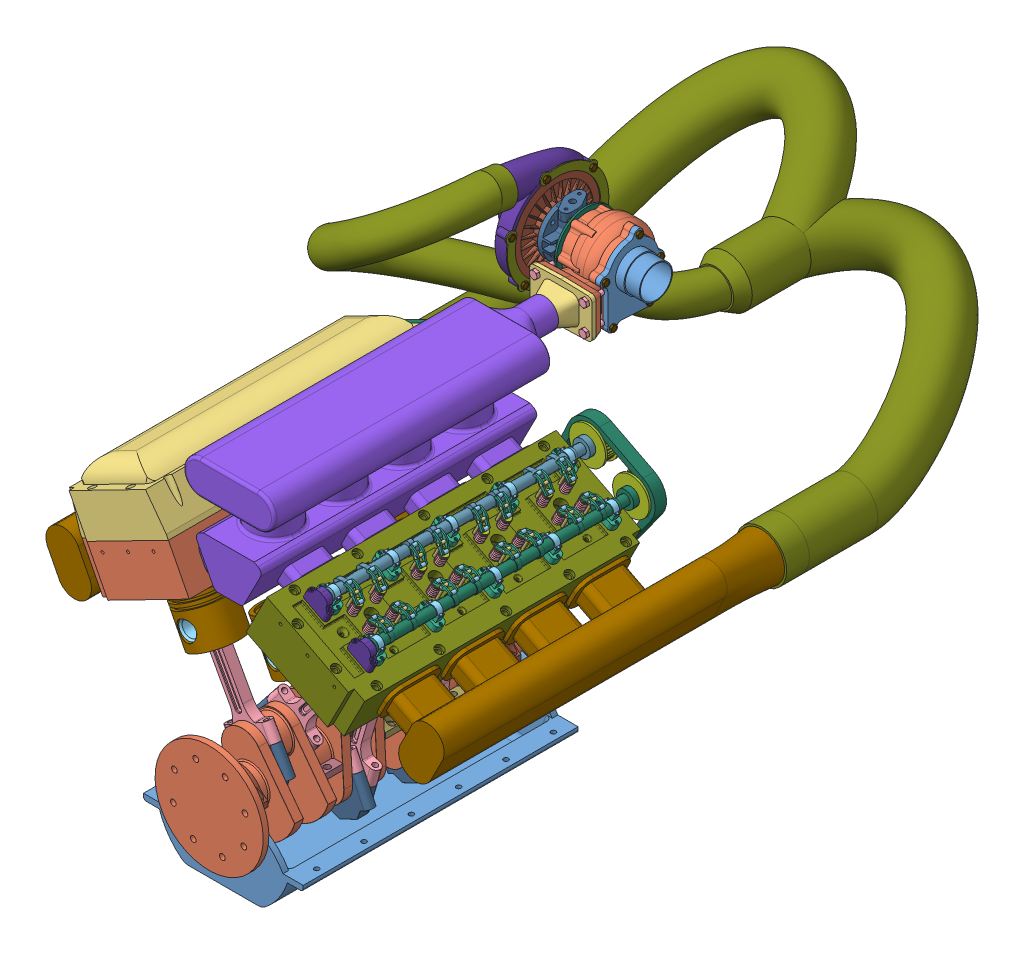
SolidWorks assembly ENSAMBLAJE DE MOTOR V8, configuration Predeterminado. Lengths in mm. (continued)
Components (placement in the parent): (continued)
- CUBIERTA DE SOPORTE DE ARBOL DE LEVAS-14: CUBIERTA DE SOPORTE DE ARBOL DE LEVAS [Predeterminado] at (198.243 212.1897 690.5) x (0.890111 -0.455744 0) z (0 0 1) size (25 9.96 10)
- SOPORTE DE ARBOL DE LEVAS-14: SOPORTE DE ARBOL DE LEVAS [Predeterminado] at (173.0848 200.3549 695.5) x (0.890111 -0.455744 0) z (0 0 1) size (40.64 22 18)
- CUBIERTA DE SOPORTE DE ARBOL DE LEVAS-15: CUBIERTA DE SOPORTE DE ARBOL DE LEVAS [Predeterminado] at (-150.1483 251.4202 398.25) x (0.890111 0.455744 0) z (0 0 1) size (25 9.96 10)
- SOPORTE DE ARBOL DE LEVAS-15: SOPORTE DE ARBOL DE LEVAS [Predeterminado] at (-155.2538 224.0901 403.25) x (0.890111 0.455744 0) z (0 0 1) size (40.64 22 18)
- CUBIERTA DE SOPORTE DE ARBOL DE LEVAS-16: CUBIERTA DE SOPORTE DE ARBOL DE LEVAS [Predeterminado] at (198.243 212.1897 587.5) x (0.890111 -0.455744 0) z (0 0 1) size (25 9.96 10)
- SOPORTE DE ARBOL DE LEVAS-16: SOPORTE DE ARBOL DE LEVAS [Predeterminado] at (173.0848 200.3549 592.5) x (0.890111 -0.455744 0) z (0 0 1) size (40.64 22 18)
- CUBIERTA DE SOPORTE DE ARBOL DE LEVAS-17: CUBIERTA DE SOPORTE DE ARBOL DE LEVAS [Predeterminado] at (121.6935 251.3837 690.5) x (0.890111 -0.455744 0) z (0 0 1) size (25 9.96 10)
- SOPORTE DE ARBOL DE LEVAS-17: SOPORTE DE ARBOL DE LEVAS [Predeterminado] at (96.5352 239.5489 695.5) x (0.890111 -0.455744 0) z (0 0 1) size (40.64 22 18)
- CUBIERTA DE SOPORTE DE ARBOL DE LEVAS-18: CUBIERTA DE SOPORTE DE ARBOL DE LEVAS [Predeterminado] at (198.243 212.1897 484.5) x (0.890111 -0.455744 0) z (0 0 1) size (25 9.96 10)
- SOPORTE DE ARBOL DE LEVAS-18: SOPORTE DE ARBOL DE LEVAS [Predeterminado] at (173.0848 200.3549 489.5) x (0.890111 -0.455744 0) z (0 0 1) size (40.64 22 18)
- CUBIERTA DE SOPORTE DE ARBOL DE LEVAS-19: CUBIERTA DE SOPORTE DE ARBOL DE LEVAS [Predeterminado] at (121.6935 251.3837 484.5) x (0.890111 -0.455744 0) z (0 0 1) size (25 9.96 10)
- SOPORTE DE ARBOL DE LEVAS-19: SOPORTE DE ARBOL DE LEVAS [Predeterminado] at (96.5352 239.5489 489.5) x (0.890111 -0.455744 0) z (0 0 1) size (40.64 22 18)
- CUBIERTA DE SOPORTE DE ARBOL DE LEVAS-20: CUBIERTA DE SOPORTE DE ARBOL DE LEVAS [Predeterminado] at (121.6935 251.3837 587.5) x (0.890111 -0.455744 0) z (0 0 1) size (25 9.96 10)
- SOPORTE DE ARBOL DE LEVAS-20: SOPORTE DE ARBOL DE LEVAS [Predeterminado] at (96.5352 239.5489 592.5) x (0.890111 -0.455744 0) z (0 0 1) size (40.64 22 18)
- CUBIERTA DE SOPORTE DE ARBOL DE LEVAS-21: CUBIERTA DE SOPORTE DE ARBOL DE LEVAS [Predeterminado] at (198.243 212.1897 278.5) x (0.890111 -0.455744 0) z (0 0 1) size (25 9.96 10)
- SOPORTE DE ARBOL DE LEVAS-21: SOPORTE DE ARBOL DE LEVAS [Predeterminado] at (173.0848 200.3549 283.5) x (0.890111 -0.455744 0) z (0 0 1) size (40.64 22 18)
- CUBIERTA DE SOPORTE DE ARBOL DE LEVAS-22: CUBIERTA DE SOPORTE DE ARBOL DE LEVAS [Predeterminado] at (198.243 212.1897 381.5) x (0.890111 -0.455744 0) z (0 0 1) size (25 9.96 10)
- SOPORTE DE ARBOL DE LEVAS-22: SOPORTE DE ARBOL DE LEVAS [Predeterminado] at (173.0848 200.3549 386.5) x (0.890111 -0.455744 0) z (0 0 1) size (40.64 22 18)
- CUBIERTA DE SOPORTE DE ARBOL DE LEVAS-23: CUBIERTA DE SOPORTE DE ARBOL DE LEVAS [Predeterminado] at (121.6935 251.3837 381.5) x (0.890111 -0.455744 0) z (0 0 1) size (25 9.96 10)
- SOPORTE DE ARBOL DE LEVAS-23: SOPORTE DE ARBOL DE LEVAS [Predeterminado] at (96.5352 239.5489 386.5) x (0.890111 -0.455744 0) z (0 0 1) size (40.64 22 18)
- CUBIERTA DE SOPORTE DE ARBOL DE LEVAS-24: CUBIERTA DE SOPORTE DE ARBOL DE LEVAS [Predeterminado] at (121.6935 251.3837 278.5) x (0.890111 -0.455744 0) z (0 0 1) size (25 9.96 10)
- SOPORTE DE ARBOL DE LEVAS-24: SOPORTE DE ARBOL DE LEVAS [Predeterminado] at (96.5352 239.5489 283.5) x (0.890111 -0.455744 0) z (0 0 1) size (40.64 22 18)
- CUBIERTA DE SOPORTE DE ARBOL DE LEVAS-25: CUBIERTA DE SOPORTE DE ARBOL DE LEVAS [Predeterminado] at (-150.1483 251.4202 612.25) x (0.890111 0.455744 0) z (0 0 1) size (25 9.96 10)
- SOPORTE DE ARBOL DE LEVAS-25: SOPORTE DE ARBOL DE LEVAS [Predeterminado] at (-155.2538 224.0901 617.25) x (0.890111 0.455744 0) z (0 0 1) size (40.64 22 18)
- CUBIERTA DE SOPORTE DE ARBOL DE LEVAS-26: CUBIERTA DE SOPORTE DE ARBOL DE LEVAS [Predeterminado] at (-150.1483 251.4202 291.25) x (0.890111 0.455744 0) z (0 0 1) size (25 9.96 10)
- SOPORTE DE ARBOL DE LEVAS-26: SOPORTE DE ARBOL DE LEVAS [Predeterminado] at (-231.8033 184.8961 617.25) x (0.890111 0.455744 0) z (0 0 1) size (40.64 22 18)
- CUBIERTA DE SOPORTE DE ARBOL DE LEVAS-27: CUBIERTA DE SOPORTE DE ARBOL DE LEVAS [Predeterminado] at (-226.6978 212.2262 612.25) x (0.890111 0.455744 0) z (0 0 1) size (25 9.96 10)
- SOPORTE DE ARBOL DE LEVAS-27: SOPORTE DE ARBOL DE LEVAS [Predeterminado] at (-155.2538 224.0901 716.25) x (0.890111 0.455744 0) z (0 0 1) size (40.64 22 18)
- CUBIERTA DE SOPORTE DE ARBOL DE LEVAS-28: CUBIERTA DE SOPORTE DE ARBOL DE LEVAS [Predeterminado] at (-226.6978 212.2262 505.25) x (0.890111 0.455744 0) z (0 0 1) size (25 9.96 10)
- SOPORTE DE ARBOL DE LEVAS-28: SOPORTE DE ARBOL DE LEVAS [Predeterminado] at (-231.8033 184.8961 510.25) x (0.890111 0.455744 0) z (0 0 1) size (40.64 22 18)
- CUBIERTA DE SOPORTE DE ARBOL DE LEVAS-29: CUBIERTA DE SOPORTE DE ARBOL DE LEVAS [Predeterminado] at (-226.6978 212.2262 711.25) x (0.890111 0.455744 0) z (0 0 1) size (25 9.96 10)
- SOPORTE DE ARBOL DE LEVAS-29: SOPORTE DE ARBOL DE LEVAS [Predeterminado] at (-231.8033 184.8961 716.25) x (0.890111 0.455744 0) z (0 0 1) size (40.64 22 18)
- CUBIERTA DE SOPORTE DE ARBOL DE LEVAS-30: CUBIERTA DE SOPORTE DE ARBOL DE LEVAS [Predeterminado] at (-150.1483 251.4202 505.25) x (0.890111 0.455744 0) z (0 0 1) size (25 9.96 10)
- SOPORTE DE ARBOL DE LEVAS-30: SOPORTE DE ARBOL DE LEVAS [Predeterminado] at (-155.2538 224.0901 510.25) x (0.890111 0.455744 0) z (0 0 1) size (40.64 22 18)
- CUBIERTA DE SOPORTE DE ARBOL DE LEVAS-31: CUBIERTA DE SOPORTE DE ARBOL DE LEVAS [Predeterminado] at (-150.1483 251.4202 711.25) x (0.890111 0.455744 0) z (0 0 1) size (25 9.96 10)
- SOPORTE DE ARBOL DE LEVAS-31: SOPORTE DE ARBOL DE LEVAS [Predeterminado] at (-155.2538 224.0901 296.25) x (0.890111 0.455744 0) z (0 0 1) size (40.64 22 18)
- CUBIERTA DE SOPORTE DE ARBOL DE LEVAS-32: CUBIERTA DE SOPORTE DE ARBOL DE LEVAS [Predeterminado] at (-226.6978 212.2262 291.25) x (0.890111 0.455744 0) z (0 0 1) size (25 9.96 10)
- SOPORTE DE ARBOL DE LEVAS-32: SOPORTE DE ARBOL DE LEVAS [Predeterminado] at (-231.8033 184.8961 296.25) x (0.890111 0.455744 0) z (0 0 1) size (40.64 22 18)
- CUBIERTA DE SOPORTE DE ARBOL DE LEVAS-33: CUBIERTA DE SOPORTE DE ARBOL DE LEVAS [Predeterminado] at (-226.6978 212.2262 398.25) x (0.890111 0.455744 0) z (0 0 1) size (25 9.96 10)
- SOPORTE DE ARBOL DE LEVAS-33: SOPORTE DE ARBOL DE LEVAS [Predeterminado] at (-231.8033 184.8961 403.25) x (0.890111 0.455744 0) z (0 0 1) size (40.64 22 18)
- ENGRANE ARBOL DE LEVAS-1: ENGRANE ARBOL DE LEVAS [Predeterminado] at (198.243 212.1897 225) x (0.628385 0.777902 0) z (0 0 1) size (64 64 27)
- ENGRANE CIGUEÑAL-1: ENGRANE CIGUEÑAL [Predeterminado] at (-14.263 -103.8973 245) x (0.937671 0.347525 0) z (0 0 -1) size (30 30 27)
- ENGRANE ARBOL DE LEVAS-2: ENGRANE ARBOL DE LEVAS [Predeterminado] at (121.6935 251.3837 225) x (0.282857 0.959162 0) z (0 0 1) size (64 64 27)
- ENGRANE ARBOL DE LEVAS-3: ENGRANE ARBOL DE LEVAS [Predeterminado] at (-150.1483 251.4202 225) x (-0.43783 0.899058 0) z (0 0 1) size (64 64 27)
- ENGRANE ARBOL DE LEVAS-4: ENGRANE ARBOL DE LEVAS [Predeterminado] at (-226.6978 212.2262 225) x (0.028509 0.999594 0) z (0 0 1) size (64 64 27)
- TORNILLO CABEZA HEXAGONAL_ENGRANE DE ARBOL DE LEVAS-1: TORNILLO CABEZA HEXAGONAL_ENGRANE DE ARBOL DE LEVAS [Predeterminado] at (198.243 212.1897 221.5) size (18 18 59)
- TORNILLO CABEZA HEXAGONAL_ENGRANE DE ARBOL DE LEVAS-2: TORNILLO CABEZA HEXAGONAL_ENGRANE DE ARBOL DE LEVAS [Predeterminado] at (121.6935 251.3837 221.5) size (18 18 59)
- TORNILLO CABEZA HEXAGONAL_ENGRANE DE ARBOL DE LEVAS-3: TORNILLO CABEZA HEXAGONAL_ENGRANE DE ARBOL DE LEVAS [Predeterminado] at (-226.6978 212.2262 221.5) size (18 18 59)
- TORNILLO CABEZA HEXAGONAL_ENGRANE DE ARBOL DE LEVAS-4: TORNILLO CABEZA HEXAGONAL_ENGRANE DE ARBOL DE LEVAS [Predeterminado] at (-150.1483 251.4202 221.5) size (18 18 59)
- TORNILLO CABEZA HEXAGONAL_ENGRANE DE ARBOL DE CIGÜEÑAL-1: TORNILLO CABEZA HEXAGONAL_ENGRANE DE ARBOL DE CIGÜEÑAL [Predeterminado] at (-14.263 -103.8973 221.5) size (20 20 38)
- SOPORTE DE RODAMIENTO PARA LA BANDA-1: SOPORTE DE RODAMIENTO PARA LA BANDA [Predeterminado] at (-14.263 120.8016 248.5) x (0.866025 -0.5 0) z (0 0 1) size (80 80 35.5)
- PERNO HEXAGONAL HUECO_PARA SOPORTE DE RODAMIENTO DE BANDA-1: PERNO HEXAGONAL HUECO_PARA SOPORTE DE RODAMIENTO DE BANDA [Predeterminado] at (7.3876 133.3016 253.5) x (-0.923728 -0.383049 0) z (0 0 -1) size (17.8 17.8 27.6)
- PERNO HEXAGONAL HUECO_PARA SOPORTE DE RODAMIENTO DE BANDA-2: PERNO HEXAGONAL HUECO_PARA SOPORTE DE RODAMIENTO DE BANDA [Predeterminado] at (7.3876 108.3016 253.5) x (-0.793594 0.608447 0) z (0 0 -1) size (17.8 17.8 27.6)
- PERNO HEXAGONAL HUECO_PARA SOPORTE DE RODAMIENTO DE BANDA-3: PERNO HEXAGONAL HUECO_PARA SOPORTE DE RODAMIENTO DE BANDA [Predeterminado] at (-14.263 95.8016 253.5) x (0.130134 0.991496 0) z (0 0 -1) size (17.8 17.8 27.6)
- PERNO HEXAGONAL HUECO_PARA SOPORTE DE RODAMIENTO DE BANDA-4: PERNO HEXAGONAL HUECO_PARA SOPORTE DE RODAMIENTO DE BANDA [Predeterminado] at (-35.9136 108.3016 253.5) x (0.923728 0.383049 0) z (0 0 -1) size (17.8 17.8 27.6)
- PERNO HEXAGONAL HUECO_PARA SOPORTE DE RODAMIENTO DE BANDA-5: PERNO HEXAGONAL HUECO_PARA SOPORTE DE RODAMIENTO DE BANDA [Predeterminado] at (-35.9136 133.3016 253.5) x (0.793594 -0.608447 0) z (0 0 -1) size (17.8 17.8 27.6)
- PERNO HEXAGONAL HUECO_PARA SOPORTE DE RODAMIENTO DE BANDA-6: PERNO HEXAGONAL HUECO_PARA SOPORTE DE RODAMIENTO DE BANDA [Predeterminado] at (-14.263 145.8016 253.5) x (-0.130134 -0.991496 0) z (0 0 -1) size (17.8 17.8 27.6)
- RODAMIENTO DE BANDA-1: RODAMIENTO DE BANDA [Predeterminado] at (-14.263 120.8016 228.5) size (55 55 24.5)
- TORNILLO CABEZA HEXAGONAL_RODAMIENTO-1: TORNILLO CABEZA HEXAGONAL_RODAMIENTO [Predeterminado] at (-14.263 120.8016 224) size (20 20 19)
- BANDA DE DISTRIBUCIÓN-1: BANDA DE DISTRIBUCIÓN [Predeterminado] at (-14.2352 120.7828 235) x (1 -0.000086 0) z (0 0 1) size (502.94 419.82 20)
- RECOLECTOR DE GASES DE ESCAPE-2: RECOLECTOR DE GASES DE ESCAPE [Predeterminado] at origin size (704.57 462.45 809.42)
Mates (geometry in assembly coordinates):
- Concéntrica1: concentric: cylinder of CIGUEÑAL-1 through (-14.263 -103.8973 253.5) axis (0 0 1) radius 32; cylinder of ? through (-14.263 -103.8973 278.5) axis (0 0 -1) radius 32
- Concéntrica9: concentric: cylinder of ? through (-29.5541 -62.6398 627.75) axis (0 0 -1) radius 33; cylinder of COJINETE SUPERIOR-1 through (-29.5541 -62.6398 627.75) axis (0 0 -1) radius 33
- Coincidente2: coincident: plane of ? through (76.4856 71.7664 609.75) normal (0 0 -1); plane of COJINETE SUPERIOR-1 through (-29.5541 -62.6398 609.75) normal (0 0 -1)
- Concéntrica10: concentric: cylinder of ? through (-29.5541 -62.6398 627.75) axis (0 0 -1) radius 33; cylinder of COJINETE INFERIOR-1 through (-29.5541 -62.6398 609.75) axis (0 0 1) radius 32
- Coincidente3: coincident: plane of assembly; plane of assembly; plane of COJINETE INFERIOR-1 through (-0.1804 -77.6794 609.75) normal (-0.455744 -0.890111 0); plane of COJINETE SUPERIOR-1 through (-58.0376 -48.056 627.75) normal (0.455744 0.890111 0)
- Coincidente4: coincident: plane of ? through (76.4856 71.7664 627.75) normal (0 0 1); plane of COJINETE INFERIOR-1 through (-29.5541 -62.6398 627.75) normal (0 0 1)
- Concéntrica11: concentric: cylinder of ? through (76.4856 71.7664 637.75) axis (0 0 -1) radius 17.8; cylinder of COJINETE-1 through (76.4856 71.7664 635.25) axis (0 0 -1) radius 17.8
- Ancho1: width: plane of ? through (76.4856 71.7664 599.75) normal (0 0 -1); plane of ? through (76.4856 71.7664 637.75) normal (0 0 1); plane of COJINETE-1 through (76.4856 71.7664 602.25) normal (0 0 -1); plane of COJINETE-1 through (76.4856 71.7664 635.25) normal (0 0 1)
- Concéntrica12: concentric: cylinder of ? through (76.4856 71.7664 656.65) axis (0 0 -1) radius 16.9; cylinder of COJINETE-1 through (76.4856 71.7664 635.25) axis (0 0 -1) radius 16.9
- Concéntrica13: concentric: cylinder of ? through (84.7286 82.2145 618.75) axis (0.61939 0.785083 0) radius 1.25; cylinder of ? through (74.0699 68.7046 618.75) axis (0.61939 0.785083 0) radius 6.3
- Concéntrica14: concentric: cylinder of ? through (76.4856 71.7664 656.65) axis (0 0 -1) radius 16.9; cylinder of PISTÓN-1 through (76.4856 71.7664 654.5) axis (0 0 -1) radius 16.9
- Ancho2: width: plane of PISTÓN-1 through (67.3727 111.2594 599.75) normal (0 0 1); plane of PISTÓN-1 through (67.3727 111.2594 637.75) normal (0 0 -1); plane of ? through (76.4856 71.7664 599.75) normal (0 0 -1); plane of ? through (76.4856 71.7664 637.75) normal (0 0 1)
- Concéntrica15: concentric: cylinder of assembly; cylinder of assembly; cylinder of COJINETE SUPERIOR-1 through (-29.5541 -62.6398 627.75) axis (0 0 -1) radius 33; cylinder of SOMBRERETE DE BIELA-1 through (-29.5541 -62.6398 600.25) axis (0 0 1) radius 33
- Coincidente5: coincident: plane of ? through (76.4856 71.7664 627.75) normal (0 0 1); plane of SOMBRERETE DE BIELA-1 through (-29.5541 -62.6398 627.75) normal (0 0 1)
- Coincidente6: coincident: plane of ? through (75.9097 72.2187 331.75) normal (0 0 1); plane of COJINETE INFERIOR-2 through (-29.5541 -62.6398 331.75) normal (0 0 1)
- Concéntrica16: concentric: cylinder of ? through (-29.5541 -62.6398 331.75) axis (0 0 -1) radius 33; cylinder of COJINETE INFERIOR-2 through (-29.5541 -62.6398 313.75) axis (0 0 1) radius 32
- Ancho3: width: plane of ? through (75.9097 72.2187 303.75) normal (0 0 -1); plane of ? through (75.9097 72.2187 341.75) normal (0 0 1); plane of COJINETE-2 through (75.9097 72.2187 306.25) normal (0 0 -1); plane of COJINETE-2 through (75.9097 72.2187 339.25) normal (0 0 1)
- Concéntrica17: concentric: cylinder of ? through (75.9097 72.2187 360.65) axis (0 0 -1) radius 16.9; cylinder of PISTÓN-2 through (75.9097 72.2187 358.5) axis (0 0 -1) radius 16.9
- Concéntrica18: concentric: cylinder of ? through (75.9097 72.2187 360.65) axis (0 0 -1) radius 16.9; cylinder of COJINETE-2 through (75.9097 72.2187 339.25) axis (0 0 -1) radius 16.9
- Concéntrica19: concentric: cylinder of ? through (-29.5541 -62.6398 331.75) axis (0 0 -1) radius 33; cylinder of COJINETE SUPERIOR-2 through (-29.5541 -62.6398 331.75) axis (0 0 -1) radius 33
- Concéntrica20: concentric: cylinder of ? through (84.108 82.702 322.75) axis (0.616027 0.787725 0) radius 1.25; cylinder of ? through (73.5072 69.1466 322.75) axis (0.616027 0.787725 0) radius 6.3
- Concéntrica21: concentric: cylinder of ? through (75.9097 72.2187 341.75) axis (0 0 -1) radius 17.8; cylinder of COJINETE-2 through (75.9097 72.2187 339.25) axis (0 0 -1) radius 17.8
- Ancho4: width: plane of PISTÓN-2 through (66.7969 111.7117 303.75) normal (0 0 1); plane of PISTÓN-2 through (66.7969 111.7117 341.75) normal (0 0 -1); plane of ? through (75.9097 72.2187 303.75) normal (0 0 -1); plane of ? through (75.9097 72.2187 341.75) normal (0 0 1)
- Coincidente7: coincident: plane of ? through (75.9097 72.2187 331.75) normal (0 0 1); plane of SOMBRERETE DE BIELA-2 through (-29.5541 -62.6398 331.75) normal (0 0 1)
- Coincidente8: coincident: plane of assembly; plane of assembly; plane of COJINETE INFERIOR-2 through (-0.1804 -77.6794 313.75) normal (-0.455744 -0.890111 0); plane of COJINETE SUPERIOR-2 through (-58.0376 -48.056 331.75) normal (0.455744 0.890111 0)
- Coincidente9: coincident: plane of ? through (75.9097 72.2187 313.75) normal (0 0 -1); plane of COJINETE SUPERIOR-2 through (-29.5541 -62.6398 313.75) normal (0 0 -1)
- Concéntrica22: concentric: cylinder of assembly; cylinder of assembly; cylinder of COJINETE SUPERIOR-2 through (-29.5541 -62.6398 331.75) axis (0 0 -1) radius 33; cylinder of SOMBRERETE DE BIELA-2 through (-29.5541 -62.6398 304.25) axis (0 0 1) radius 33
- Coincidente10: coincident: plane of ? through (-72.3378 9.5283 463.25) normal (0 0 1); plane of COJINETE INFERIOR-3 through (1.0281 -145.1549 463.25) normal (0 0 1)
- Concéntrica23: concentric: cylinder of ? through (1.0281 -145.1549 463.25) axis (0 0 -1) radius 33; cylinder of COJINETE INFERIOR-3 through (1.0281 -145.1549 445.25) axis (0 0 1) radius 32
- Ancho5: width: plane of ? through (-72.3378 9.5283 435.25) normal (0 0 -1); plane of ? through (-72.3378 9.5283 473.25) normal (0 0 1); plane of COJINETE-3 through (-72.3378 9.5283 437.75) normal (0 0 -1); plane of COJINETE-3 through (-72.3378 9.5283 470.75) normal (0 0 1)
- Concéntrica24: concentric: cylinder of ? through (-72.3378 9.5283 492.15) axis (0 0 -1) radius 16.9; cylinder of PISTÓN-3 through (-72.3378 9.5283 490) axis (0 0 -1) radius 16.9
- Concéntrica25: concentric: cylinder of ? through (-72.3378 9.5283 492.15) axis (0 0 -1) radius 16.9; cylinder of COJINETE-3 through (-72.3378 9.5283 470.75) axis (0 0 -1) radius 16.9
- Concéntrica26: concentric: cylinder of ? through (1.0281 -145.1549 463.25) axis (0 0 -1) radius 33; cylinder of COJINETE SUPERIOR-3 through (1.0281 -145.1549 463.25) axis (0 0 -1) radius 33
- Concéntrica27: concentric: cylinder of ? through (-78.0409 21.5527 454.25) axis (-0.428539 0.903523 0) radius 1.25; cylinder of ? through (-70.6665 6.0046 454.25) axis (-0.428539 0.903523 0) radius 6.3
- Concéntrica28: concentric: cylinder of ? through (-72.3378 9.5283 473.25) axis (0 0 -1) radius 17.8; cylinder of COJINETE-3 through (-72.3378 9.5283 470.75) axis (0 0 -1) radius 17.8
- Ancho6: width: plane of PISTÓN-3 through (-109.7068 25.2222 435.25) normal (0 0 1); plane of PISTÓN-3 through (-109.7068 25.2222 473.25) normal (0 0 -1); plane of ? through (-72.3378 9.5283 435.25) normal (0 0 -1); plane of ? through (-72.3378 9.5283 473.25) normal (0 0 1)
- Coincidente11: coincident: plane of ? through (-72.3378 9.5283 463.25) normal (0 0 1); plane of SOMBRERETE DE BIELA-3 through (1.0281 -145.1549 463.25) normal (0 0 1)
- Coincidente12: coincident: plane of assembly; plane of assembly; plane of COJINETE INFERIOR-3 through (30.4018 -130.1153 445.25) normal (0.455744 -0.890111 0); plane of COJINETE SUPERIOR-3 through (-27.4555 -159.7387 463.25) normal (-0.455744 0.890111 0)
- Concéntrica29: concentric: cylinder of assembly; cylinder of assembly; cylinder of COJINETE SUPERIOR-3 through (1.0281 -145.1549 463.25) axis (0 0 -1) radius 33; cylinder of SOMBRERETE DE BIELA-3 through (1.0281 -145.1549 435.75) axis (0 0 1) radius 33
- Coincidente14: coincident: plane of ? through (71.2823 63.1809 441.75) normal (0 0 1); plane of COJINETE INFERIOR-4 through (29.7257 -102.8988 441.75) normal (0 0 1)
- Concéntrica30: concentric: cylinder of ? through (29.7257 -102.8988 441.75) axis (0 0 -1) radius 33; cylinder of COJINETE INFERIOR-4 through (29.7257 -102.8988 423.75) axis (0 0 1) radius 32
- Ancho7: width: plane of ? through (71.2823 63.1809 413.75) normal (0 0 -1); plane of ? through (71.2823 63.1809 451.75) normal (0 0 1); plane of COJINETE-4 through (71.2823 63.1809 416.25) normal (0 0 -1); plane of COJINETE-4 through (71.2823 63.1809 449.25) normal (0 0 1)
- Concéntrica31: concentric: cylinder of ? through (71.2823 63.1809 470.65) axis (0 0 -1) radius 16.9; cylinder of PISTÓN-4 through (71.2823 63.1809 468.5) axis (0 0 -1) radius 16.9
- Concéntrica32: concentric: cylinder of ? through (71.2823 63.1809 470.65) axis (0 0 -1) radius 16.9; cylinder of COJINETE-4 through (71.2823 63.1809 449.25) axis (0 0 -1) radius 16.9
- Concéntrica33: concentric: cylinder of ? through (29.7257 -102.8988 441.75) axis (0 0 -1) radius 33; cylinder of COJINETE SUPERIOR-4 through (29.7257 -102.8988 441.75) axis (0 0 -1) radius 33
- Concéntrica34: concentric: cylinder of ? through (74.5128 76.0912 432.75) axis (0.242737 0.970092 0) radius 1.25; cylinder of ? through (70.3357 59.3976 432.75) axis (0.242737 0.970092 0) radius 6.3
- Concéntrica35: concentric: cylinder of ? through (71.2823 63.1809 451.75) axis (0 0 -1) radius 17.8; cylinder of COJINETE-4 through (71.2823 63.1809 449.25) axis (0 0 -1) radius 17.8
- Ancho8: width: plane of PISTÓN-4 through (62.1694 102.6739 413.75) normal (0 0 1); plane of PISTÓN-4 through (62.1694 102.6739 451.75) normal (0 0 -1); plane of ? through (71.2823 63.1809 413.75) normal (0 0 -1); plane of ? through (71.2823 63.1809 451.75) normal (0 0 1)
- Coincidente15: coincident: plane of ? through (71.2823 63.1809 441.75) normal (0 0 1); plane of SOMBRERETE DE BIELA-4 through (29.7257 -102.8988 441.75) normal (0 0 1)
- Coincidente16: coincident: plane of assembly; plane of assembly; plane of COJINETE INFERIOR-4 through (59.0993 -117.9384 423.75) normal (-0.455744 -0.890111 0); plane of COJINETE SUPERIOR-4 through (1.2421 -88.315 441.75) normal (0.455744 0.890111 0)
- Coincidente17: coincident: plane of ? through (71.2823 63.1809 423.75) normal (0 0 -1); plane of COJINETE SUPERIOR-4 through (29.7257 -102.8988 423.75) normal (0 0 -1)
- Concéntrica36: concentric: cylinder of assembly; cylinder of assembly; cylinder of COJINETE SUPERIOR-4 through (29.7257 -102.8988 441.75) axis (0 0 -1) radius 33; cylinder of SOMBRERETE DE BIELA-4 through (29.7257 -102.8988 414.25) axis (0 0 1) radius 33
- Coincidente18: coincident: plane of ? through (-112.163 87.3108 353.25) normal (0 0 1); plane of COJINETE INFERIOR-5 through (-29.5541 -62.6398 353.25) normal (0 0 1)
- Concéntrica37: concentric: cylinder of ? through (-29.5541 -62.6398 353.25) axis (0 0 -1) radius 33; cylinder of COJINETE INFERIOR-5 through (-29.5541 -62.6398 335.25) axis (0 0 1) radius 32
- Ancho9: width: plane of ? through (-112.163 87.3108 325.25) normal (0 0 -1); plane of ? through (-112.163 87.3108 363.25) normal (0 0 1); plane of COJINETE-5 through (-112.163 87.3108 327.75) normal (0 0 -1); plane of COJINETE-5 through (-112.163 87.3108 360.75) normal (0 0 1)
- Concéntrica38: concentric: cylinder of ? through (-112.163 87.3108 382.15) axis (0 0 -1) radius 16.9; cylinder of PISTÓN-5 through (-112.163 87.3108 380) axis (0 0 -1) radius 16.9
- Concéntrica39: concentric: cylinder of ? through (-112.163 87.3108 382.15) axis (0 0 -1) radius 16.9; cylinder of COJINETE-5 through (-112.163 87.3108 360.75) axis (0 0 -1) radius 16.9
- Concéntrica40: concentric: cylinder of ? through (-29.5541 -62.6398 353.25) axis (0 0 -1) radius 33; cylinder of COJINETE SUPERIOR-5 through (-29.5541 -62.6398 353.25) axis (0 0 -1) radius 33
- Concéntrica41: concentric: cylinder of ? through (-118.5846 98.9673 344.25) axis (-0.482529 0.87588 0) radius 1.25; cylinder of ? through (-110.2812 83.8949 344.25) axis (-0.482529 0.87588 0) radius 6.3
- Concéntrica42: concentric: cylinder of ? through (-112.163 87.3108 363.25) axis (0 0 -1) radius 17.8; cylinder of COJINETE-5 through (-112.163 87.3108 360.75) axis (0 0 -1) radius 17.8
- Ancho10: width: plane of PISTÓN-5 through (-149.532 103.0048 325.25) normal (0 0 1); plane of PISTÓN-5 through (-149.532 103.0048 363.25) normal (0 0 -1); plane of ? through (-112.163 87.3108 325.25) normal (0 0 -1); plane of ? through (-112.163 87.3108 363.25) normal (0 0 1)
- Coincidente19: coincident: plane of ? through (-112.163 87.3108 353.25) normal (0 0 1); plane of SOMBRERETE DE BIELA-5 through (-29.5541 -62.6398 353.25) normal (0 0 1)
- Coincidente20: coincident: plane of assembly; plane of assembly; plane of COJINETE INFERIOR-5 through (-0.1804 -47.6003 335.25) normal (0.455744 -0.890111 0); plane of COJINETE SUPERIOR-5 through (-58.0376 -77.2236 353.25) normal (-0.455744 0.890111 0)
- Coincidente21: coincident: plane of ? through (-112.163 87.3108 335.25) normal (0 0 -1); plane of COJINETE SUPERIOR-5 through (-29.5541 -62.6398 335.25) normal (0 0 -1)
- Concéntrica43: concentric: cylinder of assembly; cylinder of assembly; cylinder of COJINETE SUPERIOR-5 through (-29.5541 -62.6398 353.25) axis (0 0 -1) radius 33; cylinder of SOMBRERETE DE BIELA-5 through (-29.5541 -62.6398 325.75) axis (0 0 1) radius 33
- Coincidente22: coincident: plane of ? through (-72.3378 9.5283 573.25) normal (0 0 1); plane of COJINETE INFERIOR-6 through (1.0281 -145.1549 573.25) normal (0 0 1)
- Concéntrica44: concentric: cylinder of ? through (1.0281 -145.1549 573.25) axis (0 0 -1) radius 33; cylinder of COJINETE INFERIOR-6 through (1.0281 -145.1549 555.25) axis (0 0 1) radius 32
- Ancho11: width: plane of ? through (-72.3378 9.5283 545.25) normal (0 0 -1); plane of ? through (-72.3378 9.5283 583.25) normal (0 0 1); plane of COJINETE-6 through (-72.3378 9.5283 547.75) normal (0 0 -1); plane of COJINETE-6 through (-72.3378 9.5283 580.75) normal (0 0 1)
- Concéntrica45: concentric: cylinder of ? through (-72.3378 9.5283 602.15) axis (0 0 -1) radius 16.9; cylinder of PISTÓN-6 through (-72.3378 9.5283 600) axis (0 0 -1) radius 16.9
- Concéntrica46: concentric: cylinder of ? through (-72.3378 9.5283 602.15) axis (0 0 -1) radius 16.9; cylinder of COJINETE-6 through (-72.3378 9.5283 580.75) axis (0 0 -1) radius 16.9
- Concéntrica47: concentric: cylinder of ? through (1.0281 -145.1549 573.25) axis (0 0 -1) radius 33; cylinder of COJINETE SUPERIOR-6 through (1.0281 -145.1549 573.25) axis (0 0 -1) radius 33
- Concéntrica48: concentric: cylinder of ? through (-78.0409 21.5527 564.25) axis (-0.428539 0.903523 0) radius 1.25; cylinder of ? through (-70.6665 6.0046 564.25) axis (-0.428539 0.903523 0) radius 6.3
- Concéntrica49: concentric: cylinder of ? through (-72.3378 9.5283 583.25) axis (0 0 -1) radius 17.8; cylinder of COJINETE-6 through (-72.3378 9.5283 580.75) axis (0 0 -1) radius 17.8
- Ancho12: width: plane of PISTÓN-6 through (-109.7068 25.2222 545.25) normal (0 0 1); plane of PISTÓN-6 through (-109.7068 25.2222 583.25) normal (0 0 -1); plane of ? through (-72.3378 9.5283 545.25) normal (0 0 -1); plane of ? through (-72.3378 9.5283 583.25) normal (0 0 1)
- Coincidente23: coincident: plane of ? through (-72.3378 9.5283 573.25) normal (0 0 1); plane of SOMBRERETE DE BIELA-6 through (1.0281 -145.1549 573.25) normal (0 0 1)
- Coincidente24: coincident: plane of assembly; plane of assembly; plane of COJINETE INFERIOR-6 through (30.4018 -130.1153 555.25) normal (0.455744 -0.890111 0); plane of COJINETE SUPERIOR-6 through (-27.4555 -159.7387 573.25) normal (-0.455744 0.890111 0)
- Coincidente25: coincident: plane of ? through (-72.3378 9.5283 555.25) normal (0 0 -1); plane of COJINETE SUPERIOR-6 through (1.0281 -145.1549 555.25) normal (0 0 -1)
- Concéntrica50: concentric: cylinder of assembly; cylinder of assembly; cylinder of COJINETE SUPERIOR-6 through (1.0281 -145.1549 573.25) axis (0 0 -1) radius 33; cylinder of SOMBRERETE DE BIELA-6 through (1.0281 -145.1549 545.75) axis (0 0 1) radius 33
- Coincidente26: coincident: plane of ? through (48.7885 19.2483 551.75) normal (0 0 1); plane of COJINETE INFERIOR-7 through (1.0281 -145.1549 551.75) normal (0 0 1)
- Concéntrica51: concentric: cylinder of ? through (1.0281 -145.1549 551.75) axis (0 0 -1) radius 33; cylinder of COJINETE INFERIOR-7 through (1.0281 -145.1549 533.75) axis (0 0 1) radius 32
- Ancho13: width: plane of ? through (48.7885 19.2483 523.75) normal (0 0 -1); plane of ? through (48.7885 19.2483 561.75) normal (0 0 1); plane of COJINETE-7 through (48.7885 19.2483 526.25) normal (0 0 -1); plane of COJINETE-7 through (48.7885 19.2483 559.25) normal (0 0 1)
- Concéntrica52: concentric: cylinder of ? through (48.7885 19.2483 580.65) axis (0 0 -1) radius 16.9; cylinder of PISTÓN-7 through (48.7885 19.2483 578.5) axis (0 0 -1) radius 16.9
- Concéntrica53: concentric: cylinder of ? through (48.7885 19.2483 580.65) axis (0 0 -1) radius 16.9; cylinder of COJINETE-7 through (48.7885 19.2483 559.25) axis (0 0 -1) radius 16.9
- Concéntrica54: concentric: cylinder of ? through (1.0281 -145.1549 551.75) axis (0 0 -1) radius 33; cylinder of COJINETE SUPERIOR-7 through (1.0281 -145.1549 551.75) axis (0 0 -1) radius 33
- Concéntrica55: concentric: cylinder of ? through (52.5012 32.0282 542.75) axis (0.278974 0.960299 0) radius 1.25; cylinder of ? through (47.7005 15.5031 542.75) axis (0.278974 0.960299 0) radius 6.3
- Concéntrica56: concentric: cylinder of ? through (48.7885 19.2483 561.75) axis (0 0 -1) radius 17.8; cylinder of COJINETE-7 through (48.7885 19.2483 559.25) axis (0 0 -1) radius 17.8
- Ancho14: width: plane of PISTÓN-7 through (39.6756 58.7412 523.75) normal (0 0 1); plane of PISTÓN-7 through (39.6756 58.7412 561.75) normal (0 0 -1); plane of ? through (48.7885 19.2483 523.75) normal (0 0 -1); plane of ? through (48.7885 19.2483 561.75) normal (0 0 1)
- Coincidente27: coincident: plane of ? through (48.7885 19.2483 551.75) normal (0 0 1); plane of SOMBRERETE DE BIELA-7 through (1.0281 -145.1549 551.75) normal (0 0 1)
- Coincidente28: coincident: plane of assembly; plane of assembly; plane of COJINETE INFERIOR-7 through (30.4018 -160.1944 533.75) normal (-0.455744 -0.890111 0); plane of COJINETE SUPERIOR-7 through (-27.4555 -130.5711 551.75) normal (0.455744 0.890111 0)
- Coincidente29: coincident: plane of ? through (48.7885 19.2483 533.75) normal (0 0 -1); plane of COJINETE SUPERIOR-7 through (1.0281 -145.1549 533.75) normal (0 0 -1)
- Concéntrica57: concentric: cylinder of assembly; cylinder of assembly; cylinder of COJINETE SUPERIOR-7 through (1.0281 -145.1549 551.75) axis (0 0 -1) radius 33; cylinder of SOMBRERETE DE BIELA-7 through (1.0281 -145.1549 524.25) axis (0 0 1) radius 33
- Coincidente30: coincident: plane of ? through (-112.163 87.3108 685.25) normal (0 0 1); plane of COJINETE INFERIOR-8 through (-29.5541 -62.6398 685.25) normal (0 0 1)
- Concéntrica58: concentric: cylinder of ? through (-29.5541 -62.6398 685.25) axis (0 0 -1) radius 33; cylinder of COJINETE INFERIOR-8 through (-29.5541 -62.6398 667.25) axis (0 0 1) radius 32
- Ancho15: width: plane of ? through (-112.163 87.3108 657.25) normal (0 0 -1); plane of ? through (-112.163 87.3108 695.25) normal (0 0 1); plane of COJINETE-8 through (-112.163 87.3108 659.75) normal (0 0 -1); plane of COJINETE-8 through (-112.163 87.3108 692.75) normal (0 0 1)
- Concéntrica59: concentric: cylinder of ? through (-112.163 87.3108 714.15) axis (0 0 -1) radius 16.9; cylinder of PISTÓN-8 through (-112.163 87.3108 712) axis (0 0 -1) radius 16.9
- Concéntrica60: concentric: cylinder of ? through (-112.163 87.3108 714.15) axis (0 0 -1) radius 16.9; cylinder of COJINETE-8 through (-112.163 87.3108 692.75) axis (0 0 -1) radius 16.9
- Concéntrica61: concentric: cylinder of ? through (-29.5541 -62.6398 685.25) axis (0 0 -1) radius 33; cylinder of COJINETE SUPERIOR-8 through (-29.5541 -62.6398 685.25) axis (0 0 -1) radius 33
- Concéntrica62: concentric: cylinder of ? through (-118.5846 98.9673 676.25) axis (-0.482529 0.87588 0) radius 1.25; cylinder of ? through (-110.2812 83.8949 676.25) axis (-0.482529 0.87588 0) radius 6.3
- Concéntrica63: concentric: cylinder of ? through (-112.163 87.3108 695.25) axis (0 0 -1) radius 17.8; cylinder of COJINETE-8 through (-112.163 87.3108 692.75) axis (0 0 -1) radius 17.8
- Ancho16: width: plane of PISTÓN-8 through (-149.532 103.0048 657.25) normal (0 0 1); plane of PISTÓN-8 through (-149.532 103.0048 695.25) normal (0 0 -1); plane of ? through (-112.163 87.3108 657.25) normal (0 0 -1); plane of ? through (-112.163 87.3108 695.25) normal (0 0 1)
- Coincidente31: coincident: plane of ? through (-112.163 87.3108 685.25) normal (0 0 1); plane of SOMBRERETE DE BIELA-8 through (-29.5541 -62.6398 685.25) normal (0 0 1)
- Coincidente32: coincident: plane of assembly; plane of assembly; plane of COJINETE INFERIOR-8 through (-0.1804 -47.6003 667.25) normal (0.455744 -0.890111 0); plane of COJINETE SUPERIOR-8 through (-58.0376 -77.2236 685.25) normal (-0.455744 0.890111 0)
- Coincidente33: coincident: plane of ? through (-112.163 87.3108 667.25) normal (0 0 -1); plane of COJINETE SUPERIOR-8 through (-29.5541 -62.6398 667.25) normal (0 0 -1)
- Concéntrica64: concentric: cylinder of assembly; cylinder of assembly; cylinder of COJINETE SUPERIOR-8 through (-29.5541 -62.6398 685.25) axis (0 0 -1) radius 33; cylinder of SOMBRERETE DE BIELA-8 through (-29.5541 -62.6398 657.75) axis (0 0 1) radius 33
- Concéntrica66: concentric: cylinder of assembly; cylinder of assembly; cylinder of CIGUEÑAL-1 through (-29.5541 -62.6398 644) axis (0 0 1) radius 32; cylinder of COJINETE SUPERIOR-1 through (-29.5541 -62.6398 627.75) axis (0 0 -1) radius 32
- Concéntrica67: concentric: cylinder of ? through (-62.6634 -9.3667 676.25) axis (-0.455744 0.890111 0) radius 42.9; cylinder of PISTÓN-8 through (-138.5961 138.9373 676.25) axis (0.455744 -0.890111 0) radius 43
- Concéntrica68: concentric: cylinder of assembly; cylinder of assembly; cylinder of CIGUEÑAL-1 through (-29.5541 -62.6398 644) axis (0 0 1) radius 32; cylinder of COJINETE SUPERIOR-8 through (-29.5541 -62.6398 685.25) axis (0 0 -1) radius 32
- Concéntrica69: concentric: cylinder of PISTÓN-7 through (75.2216 70.8747 542.75) axis (-0.455744 -0.890111 0) radius 43; cylinder of ? through (34.1374 -9.3667 542.75) axis (0.455744 0.890111 0) radius 42.9
- Concéntrica71: concentric: cylinder of ? through (-62.6634 -9.3667 564.25) axis (-0.455744 0.890111 0) radius 42.9; cylinder of PISTÓN-6 through (-98.7709 61.1548 564.25) axis (0.455744 -0.890111 0) radius 43
- Concéntrica72: concentric: cylinder of assembly; cylinder of assembly; cylinder of CIGUEÑAL-1 through (1.0281 -145.1549 532) axis (0 0 1) radius 32; cylinder of COJINETE INFERIOR-6 through (1.0281 -145.1549 555.25) axis (0 0 1) radius 32
- Concéntrica73: concentric: cylinder of ? through (34.1374 -9.3667 432.75) axis (0.455744 0.890111 0) radius 42.9; cylinder of PISTÓN-4 through (97.7155 114.8074 432.75) axis (-0.455744 -0.890111 0) radius 43
- Concéntrica75: concentric: cylinder of ? through (-62.6634 -9.3667 454.25) axis (-0.455744 0.890111 0) radius 42.9; cylinder of PISTÓN-3 through (-98.7709 61.1548 454.25) axis (0.455744 -0.890111 0) radius 43
- Concéntrica76: concentric: cylinder of assembly; cylinder of assembly; cylinder of CIGUEÑAL-1 through (1.0281 -145.1549 422) axis (0 0 1) radius 32; cylinder of COJINETE SUPERIOR-3 through (1.0281 -145.1549 463.25) axis (0 0 -1) radius 32
- Concéntrica77: concentric: cylinder of ? through (34.1374 -9.3667 322.75) axis (0.455744 0.890111 0) radius 42.9; cylinder of PISTÓN-2 through (102.3429 123.8451 322.75) axis (-0.455744 -0.890111 0) radius 43
- Concéntrica79: concentric: cylinder of ? through (-62.6634 -9.3667 344.25) axis (-0.455744 0.890111 0) radius 42.9; cylinder of PISTÓN-5 through (-138.5961 138.9373 344.25) axis (0.455744 -0.890111 0) radius 43
- Concéntrica80: concentric: cylinder of assembly; cylinder of assembly; cylinder of CIGUEÑAL-1 through (-29.5541 -62.6398 312) axis (0 0 1) radius 32; cylinder of COJINETE INFERIOR-5 through (-29.5541 -62.6398 335.25) axis (0 0 1) radius 32
- Coincidente34: coincident: plane of ? through (-1.196 -84.8168 322.75) normal (-0.616027 -0.787725 0); plane of SOMBRERETE DE BIELA-2 through (-57.9122 -40.4629 322.75) normal (0.616027 0.787725 0)
- Coincidente35: coincident: plane of ? through (1.9776 -45.2688 344.25) normal (0.482529 -0.87588 0); plane of SOMBRERETE DE BIELA-5 through (-61.0858 -80.0109 344.25) normal (-0.482529 0.87588 0)
- Coincidente36: coincident: plane of ? through (-31.4987 -160.5823 454.25) normal (0.428539 -0.903523 0); plane of SOMBRERETE DE BIELA-3 through (-31.4987 -160.5823 454.25) normal (-0.428539 0.903523 0)
- Coincidente37: coincident: plane of ? through (64.649 -111.6374 432.75) normal (-0.242737 -0.970092 0); plane of SOMBRERETE DE BIELA-4 through (-5.1976 -94.1603 432.75) normal (0.242737 0.970092 0)
- Coincidente38: coincident: plane of ? through (35.5988 -155.1979 542.75) normal (-0.278974 -0.960299 0); plane of SOMBRERETE DE BIELA-7 through (-33.5427 -135.1118 542.75) normal (0.278974 0.960299 0)
- Coincidente39: coincident: plane of ? through (33.5549 -129.7275 564.25) normal (0.428539 -0.903523 0); plane of SOMBRERETE DE BIELA-6 through (-31.4987 -160.5823 564.25) normal (-0.428539 0.903523 0)
- Coincidente40: coincident: plane of ? through (-1.2911 -84.9379 618.75) normal (-0.61939 -0.785083 0); plane of SOMBRERETE DE BIELA-1 through (-57.8171 -40.3418 618.75) normal (0.61939 0.785083 0)
- Coincidente41: coincident: plane of ? through (1.9776 -45.2688 676.25) normal (0.482529 -0.87588 0); plane of SOMBRERETE DE BIELA-8 through (-61.0858 -80.0109 676.25) normal (-0.482529 0.87588 0)
- Concéntrica81: concentric: cylinder of assembly; cylinder of assembly; cylinder of CIGUEÑAL-1 through (-14.263 -103.8973 590.5) axis (0 0 1) radius 32; cylinder of SEGURO DE CIGÜEÑAL DE 38mm-1 through (-14.263 -103.8973 590.5) axis (0 0 1) radius 32
- Concéntrica82: concentric: cylinder of ? through (26.737 -103.8973 609.5) axis (0 -1 0) radius 5.5; cylinder of SEGURO DE CIGÜEÑAL DE 38mm-1 through (26.737 -149.8973 609.5) axis (0 1 0) radius 7.5
- Concéntrica83: concentric: cylinder of assembly; cylinder of assembly; cylinder of CIGUEÑAL-1 through (-14.263 -103.8973 480.5) axis (0 0 1) radius 32; cylinder of SEGURO DE CIGÜEÑAL DE 36mm-1 through (-14.263 -103.8973 516.5) axis (0 0 -1) radius 32
- Concéntrica84: concentric: cylinder of ? through (-55.263 -103.8973 498.5) axis (0 -1 0) radius 5.5; cylinder of SEGURO DE CIGÜEÑAL DE 36mm-1 through (-55.263 -57.8973 498.5) axis (0 -1 0) radius 7.5
- Concéntrica85: concentric: cylinder of assembly; cylinder of assembly; cylinder of CIGUEÑAL-1 through (-14.263 -103.8973 740.5) axis (0 0 -1) radius 32; cylinder of SEGURO DE CIGÜEÑAL DE 18mm-1 through (-14.263 -103.8973 722.5) axis (0 0 1) radius 32
- Concéntrica86: concentric: cylinder of ? through (26.737 -103.8973 731.5) axis (0 -1 0) radius 5.5; cylinder of SEGURO DE CIGÜEÑAL DE 18mm-1 through (26.737 -93.8973 731.5) axis (0 1 0) radius 5.5
- Concéntrica87: concentric: cylinder of assembly; cylinder of assembly; cylinder of CIGUEÑAL-1 through (-14.263 -103.8973 370.5) axis (0 0 1) radius 32; cylinder of SEGURO DE CIGÜEÑAL DE 36mm-2 through (-14.263 -103.8973 370.5) axis (0 0 1) radius 42
- Concéntrica88: concentric: cylinder of ? through (26.737 -103.8973 388.5) axis (0 -1 0) radius 5.5; cylinder of SEGURO DE CIGÜEÑAL DE 36mm-2 through (26.737 -149.8973 388.5) axis (0 1 0) radius 7.5
- Concéntrica89: concentric: cylinder of assembly; cylinder of assembly; cylinder of CIGUEÑAL-1 through (-14.263 -103.8973 253.5) axis (0 0 1) radius 32; cylinder of SEGURO DE CIGÜEÑAL DE 18mm-2 through (-14.263 -103.8973 278.5) axis (0 0 1) radius 42
- Concéntrica90: concentric: cylinder of ? through (26.737 -103.8973 287.5) axis (0 -1 0) radius 5.5; cylinder of SEGURO DE CIGÜEÑAL DE 18mm-2 through (26.737 -57.8973 287.5) axis (0 -1 0) radius 7.5
- Coincidente43: coincident: plane of ? through (-129.263 -163.8973 760.5) normal (0 0 1); plane of CULATA_IZQUIERDO-2 through (72.1996 252.0089 760.5) normal (0 0 1)
- Coincidente44: coincident: plane of ? through (44.8393 176.1412 750.5) normal (0.455744 0.890111 0); plane of CULATA_IZQUIERDO-2 through (178.4783 107.717 760.5) normal (-0.455744 -0.890111 0)
- Concéntrica92: concentric: cylinder of ? through (188.2384 102.7198 720.5) axis (0.455744 0.890111 0) radius 5.25; cylinder of CULATA_IZQUIERDO-2 through (224.6979 173.9287 720.5) axis (0.455744 0.890111 0) radius 5.25
- Coincidente66: coincident: plane of assembly; plane of assembly; plane of CULATA_IZQUIERDO-2 through (214.9378 178.9259 760.5) normal (0.455744 0.890111 0); plane of SOPORTE EXTERNO DE ARBOL DE LEVAS-2 through (168.1892 202.8615 713.5) normal (-0.455744 -0.890111 0)
- Concéntrica134: concentric: cylinder of assembly; cylinder of assembly; cylinder of CULATA_IZQUIERDO-2 through (203.3486 184.8597 713) axis (0.455744 0.890111 0) radius 2.25; cylinder of SOPORTE EXTERNO DE ARBOL DE LEVAS-2 through (211.0962 199.9916 713) axis (0.455744 0.890111 0) radius 2.25
- Concéntrica135: concentric: cylinder of assembly; cylinder of assembly; cylinder of CULATA_IZQUIERDO-2 through (173.0848 200.3549 713) axis (0.455744 0.890111 0) radius 2.25; cylinder of SOPORTE EXTERNO DE ARBOL DE LEVAS-2 through (180.8324 215.4868 713) axis (0.455744 0.890111 0) radius 2.25
- Coincidente68: coincident: plane of assembly; plane of assembly; plane of CULATA_IZQUIERDO-2 through (214.9378 178.9259 760.5) normal (0.455744 0.890111 0); plane of SOPORTE EXTERNO DE ARBOL DE LEVAS-1 through (91.6396 242.0555 713.5) normal (-0.455744 -0.890111 0)
- Concéntrica136: concentric: cylinder of assembly; cylinder of assembly; cylinder of CULATA_IZQUIERDO-2 through (126.799 224.0536 713) axis (0.455744 0.890111 0) radius 2.25; cylinder of SOPORTE EXTERNO DE ARBOL DE LEVAS-1 through (134.5467 239.1855 713) axis (0.455744 0.890111 0) radius 3
- Concéntrica137: concentric: cylinder of assembly; cylinder of assembly; cylinder of CULATA_IZQUIERDO-2 through (96.5352 239.5489 713) axis (0.455744 0.890111 0) radius 2.25; cylinder of SOPORTE EXTERNO DE ARBOL DE LEVAS-1 through (104.2829 254.6808 713) axis (0.455744 0.890111 0) radius 2.25
- Coincidente69: coincident: plane of assembly; plane of assembly; plane of CULATA_DERECHO-1 through (-100.6544 252.0454 253.5) normal (-0.455744 0.890111 0); plane of SOPORTE EXTERNO DE ARBOL DE LEVAS-4 through (-160.1494 221.5835 734.25) normal (0.455744 -0.890111 0)
- Concéntrica138: concentric: cylinder of assembly; cylinder of assembly; cylinder of CULATA_DERECHO-1 through (-124.99 239.5854 733.75) axis (-0.455744 0.890111 0) radius 2.25; cylinder of SOPORTE EXTERNO DE ARBOL DE LEVAS-4 through (-132.7376 254.7172 733.75) axis (-0.455744 0.890111 0) radius 3
- Concéntrica139: concentric: cylinder of assembly; cylinder of assembly; cylinder of CULATA_DERECHO-1 through (-155.2538 224.0901 733.75) axis (-0.455744 0.890111 0) radius 2.25; cylinder of SOPORTE EXTERNO DE ARBOL DE LEVAS-4 through (-163.0014 239.222 733.75) axis (-0.455744 0.890111 0) radius 2.25
- Coincidente70: coincident: plane of assembly; plane of assembly; plane of CULATA_DERECHO-1 through (-100.6544 252.0454 253.5) normal (-0.455744 0.890111 0); plane of SOPORTE EXTERNO DE ARBOL DE LEVAS-3 through (-236.699 182.3895 734.25) normal (0.455744 -0.890111 0)
- Concéntrica140: concentric: cylinder of assembly; cylinder of assembly; cylinder of CULATA_DERECHO-1 through (-201.5396 200.3914 733.75) axis (-0.455744 0.890111 0) radius 2.25; cylinder of SOPORTE EXTERNO DE ARBOL DE LEVAS-3 through (-209.2872 215.5233 733.75) axis (-0.455744 0.890111 0) radius 3
- Concéntrica141: concentric: cylinder of assembly; cylinder of assembly; cylinder of CULATA_DERECHO-1 through (-231.8033 184.8961 733.75) axis (-0.455744 0.890111 0) radius 2.25; cylinder of SOPORTE EXTERNO DE ARBOL DE LEVAS-3 through (-239.551 200.028 733.75) axis (-0.455744 0.890111 0) radius 2.25
- Coincidente87: coincident: plane of ? through (-255.5938 82.8388 750.5) normal (-0.455744 0.890111 0); plane of CULATA_DERECHO-1 through (-64.1949 180.8365 253.5) normal (0.455744 -0.890111 0)
- Concéntrica172: concentric: cylinder of ? through (-216.7644 102.7198 720.5) axis (-0.455744 0.890111 0) radius 5.25; cylinder of CULATA_DERECHO-1 through (-253.2239 173.9287 720.5) axis (-0.455744 0.890111 0) radius 5.25
- Paralelo2: parallel: line of ? through (-225.6256 98.1827 750.5) axis (0 0 -1); line of CULATA_DERECHO-1 through (-225.5542 98.2193 268.5) axis (0 0 1)
- Distancia límite12: limit distance = 0 mm: plane of assembly; plane of assembly; plane of CULATA_DERECHO-1 through (-140.7516 143.3241 454.25) normal (0.455744 -0.890111 0); plane of VÁLVULA-13 through (-155.9725 135.5309 474.25) normal (0.455744 -0.890111 0)
- Distancia límite9: limit distance = 0 mm: plane of assembly; plane of assembly; plane of CULATA_DERECHO-1 through (-140.7516 143.3241 564.25) normal (0.455744 -0.890111 0); plane of VÁLVULA-10 through (-155.9725 135.5309 584.25) normal (0.455744 -0.890111 0)
- Distancia límite11: limit distance = 0 mm: plane of assembly; plane of assembly; plane of CULATA_DERECHO-1 through (-140.7516 143.3241 564.25) normal (0.455744 -0.890111 0); plane of VÁLVULA-12 through (-155.9725 135.5309 544.25) normal (0.455744 -0.890111 0)
